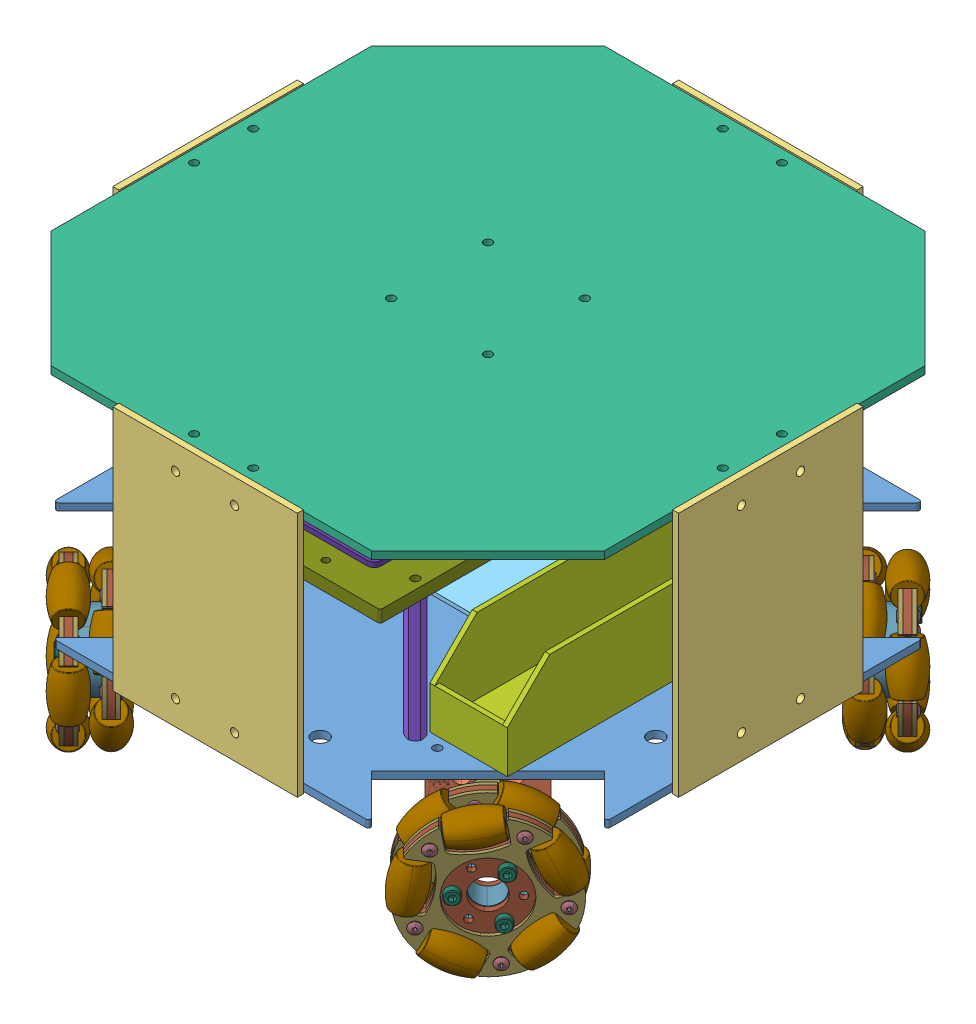
SolidWorks assembly ouijabot, configuration Default. Lengths in mm.
Overall size (259.23 176 257.62).
1225 component instances, 80 part files, 142 mates.
Components (placement in the parent):
- base-1: base [Default] at origin size (228.6 3 228.6)
- motor-mount-pololu-1995-1: motor-mount-pololu-1995 [Default] at (-74.3523 -18.4 78.9485) x (-0.707107 0 -0.707107) z (-0.707107 0 0.707107) size (36.8 36.8 6.5)
- motor-mount-pololu-1995-2: motor-mount-pololu-1995 [Default] at (-78.9485 -18.4 -74.3523) x (0.707107 0 -0.707107) z (-0.707107 0 -0.707107) size (36.8 36.8 6.5)
- motor-mount-pololu-1995-3: motor-mount-pololu-1995 [Default] at (78.9485 -18.4 74.3523) x (-0.707107 0 0.707107) z (0.707107 0 0.707107) size (36.8 36.8 6.5)
- motor-mount-pololu-1995-5: motor-mount-pololu-1995 [Default] at (74.3523 -18.4 -78.9485) x (0.707107 0 0.707107) z (0.707107 0 -0.707107) size (36.8 36.8 6.5)
- motor-pololu-2823-1: motor-pololu-2823 [Default] at (-61.3415 -18.4 33.1633) x (0.707107 0 0.707107) z (-0.707107 0 0.707107) size (36.88 41.23 90.1)
- motor-pololu-2823-2: motor-pololu-2823 [Default] at (33.1633 -18.4 61.3415) x (0.707107 0 -0.707107) z (0.707107 0 0.707107) size (36.88 41.23 90.1)
- motor-pololu-2823-3: motor-pololu-2823 [Default] at (-33.1633 -18.4 -61.3415) x (-0.707107 0 0.707107) z (-0.707107 0 -0.707107) size (36.88 41.23 90.1)
- motor-pololu-2823-4: motor-pololu-2823 [Default] at (61.3415 -18.4 -33.1633) x (-0.707107 0 -0.707107) z (0.707107 0 -0.707107) size (36.88 41.23 90.1)
- standoff-10mm-1: standoff-10mm [94868A166] at (-38 8 0) x (1 0 0) z (0 -1 0) size (4.5 5.2 10.38)
- standoff-10mm-2: standoff-10mm [94868A166] at (38 8 0) x (0.843217 0 -0.537573) z (0 -1 0) size (4.5 5.2 10.38)
- protoboard-1: protoboard [Default] at (0 13 0) size (86.36 1.6 60.96)
- angle-bracket-1: angle-bracket [Default] at (114.3 3 9.025) x (0 0 -1) z (0 1 0) size (6.35 8.71 9.53)
- angle-bracket-2: angle-bracket [Default] at (114.3 3 -15.375) x (0 0 -1) z (0 1 0) size (6.35 8.71 9.53)
- angle-bracket-4: angle-bracket [Default] at (9.025 3 -114.3) x (-1 0 0) z (0 1 0) size (6.35 8.71 9.53)
- angle-bracket-6: angle-bracket [Default] at (-15.375 3 -114.3) x (-1 0 0) z (0 1 0) size (6.35 8.71 9.53)
- angle-bracket-8: angle-bracket [Default] at (-114.3 3 -9.025) x (0 0 1) z (0 1 0) size (6.35 8.71 9.53)
- angle-bracket-10: angle-bracket [Default] at (-114.3 3 15.375) x (0 0 1) z (0 1 0) size (6.35 8.71 9.53)
- angle-bracket-12: angle-bracket [Default] at (-9.025 3 114.3) x (1 0 0) z (0 1 0) size (6.35 8.71 9.53)
- angle-bracket-14: angle-bracket [Default] at (15.375 3 114.3) x (1 0 0) z (0 1 0) size (6.35 8.71 9.53)
- battery-holder-1: battery-holder [Default] at (-65 6.1 0) size (32 35 146)
- battery-holder-2: battery-holder [Default] at (65 6.1 0) size (32 35 146)
- standoff-51mm-1: standoff-51mm [95947A075] at (-44 28.5 74) x (1 0 0) z (0 -1 0) size (6 6.93 51.34)
- standoff-51mm-2: standoff-51mm [95947A075] at (44 28.5 74) x (0.982082 0 -0.188455) z (0 -1 0) size (6 6.93 51.34)
- standoff-51mm-4: standoff-51mm [95947A075] at (44 28.5 -74) x (0.918365 0 -0.395734) z (0 -1 0) size (6 6.93 51.34)
- standoff-51mm-6: standoff-51mm [95947A075] at (-44 28.5 -74) x (0.8 0 -0.6) z (0 -1 0) size (6 6.93 51.34)
- omni-wheel-60mm-1: omni-wheel-60mm [Default] at (-82.2012 -25.4 -82.2012) x (-0.107758 0.98832 0.107758) z (-0.707107 0 -0.707107) size (78.62 80.66 25.5)
  - (Nex) [RB-Nex-75] [14145] 60mm Aluminum Omni Wheel - SolidWorks Model.STEP-1: (Nex) [RB-Nex-75] [14145] 60mm Aluminum Omni Wheel - SolidWorks Model.STEP [Default] at origin size (78.62 80.66 25.5)
    - 60mm90__5______-______________(A__ ).STEP-1: 60mm90__5______-______________(A__ ).STEP [Default] at (0 0 6.25) size (64.79 61.62 13)
      - 60mm90__5______-______________(A__).STEP-1: 60mm90__5______-______________(A__).STEP [Default] at origin size (25 13 13)
        - 60mm90__5______-______(A__).STEP-1: 60mm90__5______-______(A__).STEP [Default] at origin size (18.5 13 13)
        - 60mm90__5______-______-__(A__).STEP-1: 60mm90__5______-______-__(A__).STEP [Default] at (0 23.5 0) x (1 0 0) z (0 -0.978837 -0.204643) size (25 2.5 2.5)
      - 60mm90__5______-______________(A__).STEP-2: 60mm90__5______-______________(A__).STEP [Default] x (0.309017 -0.951057 0) z (0 0 1) size (25 13 13)
        - 60mm90__5______-______(A__).STEP-1: 60mm90__5______-______(A__).STEP [Default] at origin size (18.5 13 13)
        - 60mm90__5______-______-__(A__).STEP-1: 60mm90__5______-______-__(A__).STEP [Default] at (0 23.5 0) x (1 0 0) z (0 -0.978837 -0.204643) size (25 2.5 2.5)
      - 60mm90__5______-______________(A__).STEP-3: 60mm90__5______-______________(A__).STEP [Default] x (-0.809017 -0.587785 0) z (0 0 1) size (25 13 13)
        - 60mm90__5______-______(A__).STEP-1: 60mm90__5______-______(A__).STEP [Default] at origin size (18.5 13 13)
        - 60mm90__5______-______-__(A__).STEP-1: 60mm90__5______-______-__(A__).STEP [Default] at (0 23.5 0) x (1 0 0) z (0 -0.978837 -0.204643) size (25 2.5 2.5)
      - 60mm90__5______-______________(A__).STEP-4: 60mm90__5______-______________(A__).STEP [Default] x (-0.809017 0.587785 0) z (0 0 1) size (25 13 13)
        - 60mm90__5______-______(A__).STEP-1: 60mm90__5______-______(A__).STEP [Default] at origin size (18.5 13 13)
        - 60mm90__5______-______-__(A__).STEP-1: 60mm90__5______-______-__(A__).STEP [Default] at (0 23.5 0) x (1 0 0) z (0 -0.978837 -0.204643) size (25 2.5 2.5)
      - 60mm90__5______-______________(A__).STEP-5: 60mm90__5______-______________(A__).STEP [Default] x (0.309017 0.951057 0) z (0 0 1) size (25 13 13)
        - 60mm90__5______-______(A__).STEP-1: 60mm90__5______-______(A__).STEP [Default] at origin size (18.5 13 13)
        - 60mm90__5______-______-__(A__).STEP-1: 60mm90__5______-______-__(A__).STEP [Default] at (0 23.5 0) x (1 0 0) z (0 -0.978837 -0.204643) size (25 2.5 2.5)
      - 60mm90__5______-____________(A__).STEP-1: 60mm90__5______-____________(A__).STEP [Default] at origin size (56.91 55.07 2.5)
      - 60mm90__5______-__________(A__).STEP-1: 60mm90__5______-__________(A__).STEP [Default] at (0 0 2) size (56.91 55.07 1.5)
      - 60mm90__5______-__________(A__).STEP-2: 60mm90__5______-__________(A__).STEP [Default] at (0 0 -2) size (56.91 55.07 1.5)
      - ____3X5.STEP-1: ____3X5.STEP [Default] at (-14.1068 19.4164 -10.9942) x (1 0 0) z (0 -1 0) size (4.8 7.01 4.8)
      - ____3X5.STEP-2: ____3X5.STEP [Default] at (14.1068 19.4164 -10.9942) x (0.309017 -0.951057 0) z (-0.951057 -0.309017 0) size (4.8 7.01 4.8)
      - ____3X5.STEP-3: ____3X5.STEP [Default] at (22.8254 -7.4164 -10.9942) x (-0.809017 -0.587785 0) z (-0.587785 0.809017 0) size (4.8 7.01 4.8)
      - ____3X5.STEP-4: ____3X5.STEP [Default] at (0 -24 -10.9942) x (-0.809017 0.587785 0) z (0.587785 0.809017 0) size (4.8 7.01 4.8)
      - ____3X5.STEP-5: ____3X5.STEP [Default] at (-22.8254 -7.4164 -10.9942) x (0.309017 0.951057 0) z (0.951057 -0.309017 0) size (4.8 7.01 4.8)
    - 60mm90__5______-______________(A__ ).STEP-2: 60mm90__5______-______________(A__ ).STEP [Default] at (0 0 -6.25) x (0.309017 0.951057 0) z (0 0 -1) size (64.79 61.62 13)
      - 60mm90__5______-______________(A__).STEP-1: 60mm90__5______-______________(A__).STEP [Default] at origin size (25 13 13)
        - 60mm90__5______-______(A__).STEP-1: 60mm90__5______-______(A__).STEP [Default] at origin size (18.5 13 13)
        - 60mm90__5______-______-__(A__).STEP-1: 60mm90__5______-______-__(A__).STEP [Default] at (0 23.5 0) x (1 0 0) z (0 -0.978837 -0.204643) size (25 2.5 2.5)
      - 60mm90__5______-______________(A__).STEP-2: 60mm90__5______-______________(A__).STEP [Default] x (0.309017 -0.951057 0) z (0 0 1) size (25 13 13)
        - 60mm90__5______-______(A__).STEP-1: 60mm90__5______-______(A__).STEP [Default] at origin size (18.5 13 13)
        - 60mm90__5______-______-__(A__).STEP-1: 60mm90__5______-______-__(A__).STEP [Default] at (0 23.5 0) x (1 0 0) z (0 -0.978837 -0.204643) size (25 2.5 2.5)
      - 60mm90__5______-______________(A__).STEP-3: 60mm90__5______-______________(A__).STEP [Default] x (-0.809017 -0.587785 0) z (0 0 1) size (25 13 13)
        - 60mm90__5______-______(A__).STEP-1: 60mm90__5______-______(A__).STEP [Default] at origin size (18.5 13 13)
        - 60mm90__5______-______-__(A__).STEP-1: 60mm90__5______-______-__(A__).STEP [Default] at (0 23.5 0) x (1 0 0) z (0 -0.978837 -0.204643) size (25 2.5 2.5)
      - 60mm90__5______-______________(A__).STEP-4: 60mm90__5______-______________(A__).STEP [Default] x (-0.809017 0.587785 0) z (0 0 1) size (25 13 13)
        - 60mm90__5______-______(A__).STEP-1: 60mm90__5______-______(A__).STEP [Default] at origin size (18.5 13 13)
        - 60mm90__5______-______-__(A__).STEP-1: 60mm90__5______-______-__(A__).STEP [Default] at (0 23.5 0) x (1 0 0) z (0 -0.978837 -0.204643) size (25 2.5 2.5)
      - 60mm90__5______-______________(A__).STEP-5: 60mm90__5______-______________(A__).STEP [Default] x (0.309017 0.951057 0) z (0 0 1) size (25 13 13)
        - 60mm90__5______-______(A__).STEP-1: 60mm90__5______-______(A__).STEP [Default] at origin size (18.5 13 13)
        - 60mm90__5______-______-__(A__).STEP-1: 60mm90__5______-______-__(A__).STEP [Default] at (0 23.5 0) x (1 0 0) z (0 -0.978837 -0.204643) size (25 2.5 2.5)
      - 60mm90__5______-____________(A__).STEP-1: 60mm90__5______-____________(A__).STEP [Default] at origin size (56.91 55.07 2.5)
      - 60mm90__5______-__________(A__).STEP-1: 60mm90__5______-__________(A__).STEP [Default] at (0 0 2) size (56.91 55.07 1.5)
      - 60mm90__5______-__________(A__).STEP-2: 60mm90__5______-__________(A__).STEP [Default] at (0 0 -2) size (56.91 55.07 1.5)
      - ____3X5.STEP-1: ____3X5.STEP [Default] at (-14.1068 19.4164 -10.9942) x (1 0 0) z (0 -1 0) size (4.8 7.01 4.8)
      - ____3X5.STEP-2: ____3X5.STEP [Default] at (14.1068 19.4164 -10.9942) x (0.309017 -0.951057 0) z (-0.951057 -0.309017 0) size (4.8 7.01 4.8)
      - ____3X5.STEP-3: ____3X5.STEP [Default] at (22.8254 -7.4164 -10.9942) x (-0.809017 -0.587785 0) z (-0.587785 0.809017 0) size (4.8 7.01 4.8)
      - ____3X5.STEP-4: ____3X5.STEP [Default] at (0 -24 -10.9942) x (-0.809017 0.587785 0) z (0.587785 0.809017 0) size (4.8 7.01 4.8)
      - ____3X5.STEP-5: ____3X5.STEP [Default] at (-22.8254 -7.4164 -10.9942) x (0.309017 0.951057 0) z (0.951057 -0.309017 0) size (4.8 7.01 4.8)
    - 60mm90__5______-__________(A__)-0.STEP-1: 60mm90__5______-__________(A__)-0.STEP [Default] x (0.994522 0.104528 0) z (0 0 1) size (28 28 10)
    - __________(M3X20).STEP-1: __________(M3X20).STEP [Default] at (-1.0975 10.4425 7.5) x (0.905128 0.425139 0) z (0.425139 -0.905128 0) size (5.5 21 5.5)
    - __________(M3X20).STEP-2: __________(M3X20).STEP [Default] at (-8.4947 -6.1717 7.5) x (-0.820745 0.571294 0) z (0.571294 0.820745 0) size (5.5 21 5.5)
    - __________(M3X20).STEP-3: __________(M3X20).STEP [Default] at (9.5922 -4.2707 7.5) x (-0.084383 -0.996433 0) z (-0.996433 0.084383 0) size (5.5 21 5.5)
- omni-wheel-60mm-2: omni-wheel-60mm [Default] at (82.2012 -25.4 -82.2012) x (-0.276059 0.920643 -0.276059) z (0.707107 0 -0.707107) size (78.62 80.66 25.5)
  - (Nex) [RB-Nex-75] [14145] 60mm Aluminum Omni Wheel - SolidWorks Model.STEP-1: (Nex) [RB-Nex-75] [14145] 60mm Aluminum Omni Wheel - SolidWorks Model.STEP [Default] at origin size (78.62 80.66 25.5)
    - 60mm90__5______-______________(A__ ).STEP-1: 60mm90__5______-______________(A__ ).STEP [Default] at (0 0 6.25) size (64.79 61.62 13)
      - 60mm90__5______-______________(A__).STEP-1: 60mm90__5______-______________(A__).STEP [Default] at origin size (25 13 13)
        - 60mm90__5______-______(A__).STEP-1: 60mm90__5______-______(A__).STEP [Default] at origin size (18.5 13 13)
        - 60mm90__5______-______-__(A__).STEP-1: 60mm90__5______-______-__(A__).STEP [Default] at (0 23.5 0) x (1 0 0) z (0 -0.978837 -0.204643) size (25 2.5 2.5)
      - 60mm90__5______-______________(A__).STEP-2: 60mm90__5______-______________(A__).STEP [Default] x (0.309017 -0.951057 0) z (0 0 1) size (25 13 13)
        - 60mm90__5______-______(A__).STEP-1: 60mm90__5______-______(A__).STEP [Default] at origin size (18.5 13 13)
        - 60mm90__5______-______-__(A__).STEP-1: 60mm90__5______-______-__(A__).STEP [Default] at (0 23.5 0) x (1 0 0) z (0 -0.978837 -0.204643) size (25 2.5 2.5)
      - 60mm90__5______-______________(A__).STEP-3: 60mm90__5______-______________(A__).STEP [Default] x (-0.809017 -0.587785 0) z (0 0 1) size (25 13 13)
        - 60mm90__5______-______(A__).STEP-1: 60mm90__5______-______(A__).STEP [Default] at origin size (18.5 13 13)
        - 60mm90__5______-______-__(A__).STEP-1: 60mm90__5______-______-__(A__).STEP [Default] at (0 23.5 0) x (1 0 0) z (0 -0.978837 -0.204643) size (25 2.5 2.5)
      - 60mm90__5______-______________(A__).STEP-4: 60mm90__5______-______________(A__).STEP [Default] x (-0.809017 0.587785 0) z (0 0 1) size (25 13 13)
        - 60mm90__5______-______(A__).STEP-1: 60mm90__5______-______(A__).STEP [Default] at origin size (18.5 13 13)
        - 60mm90__5______-______-__(A__).STEP-1: 60mm90__5______-______-__(A__).STEP [Default] at (0 23.5 0) x (1 0 0) z (0 -0.978837 -0.204643) size (25 2.5 2.5)
      - 60mm90__5______-______________(A__).STEP-5: 60mm90__5______-______________(A__).STEP [Default] x (0.309017 0.951057 0) z (0 0 1) size (25 13 13)
        - 60mm90__5______-______(A__).STEP-1: 60mm90__5______-______(A__).STEP [Default] at origin size (18.5 13 13)
        - 60mm90__5______-______-__(A__).STEP-1: 60mm90__5______-______-__(A__).STEP [Default] at (0 23.5 0) x (1 0 0) z (0 -0.978837 -0.204643) size (25 2.5 2.5)
      - 60mm90__5______-____________(A__).STEP-1: 60mm90__5______-____________(A__).STEP [Default] at origin size (56.91 55.07 2.5)
      - 60mm90__5______-__________(A__).STEP-1: 60mm90__5______-__________(A__).STEP [Default] at (0 0 2) size (56.91 55.07 1.5)
      - 60mm90__5______-__________(A__).STEP-2: 60mm90__5______-__________(A__).STEP [Default] at (0 0 -2) size (56.91 55.07 1.5)
      - ____3X5.STEP-1: ____3X5.STEP [Default] at (-14.1068 19.4164 -10.9942) x (1 0 0) z (0 -1 0) size (4.8 7.01 4.8)
      - ____3X5.STEP-2: ____3X5.STEP [Default] at (14.1068 19.4164 -10.9942) x (0.309017 -0.951057 0) z (-0.951057 -0.309017 0) size (4.8 7.01 4.8)
      - ____3X5.STEP-3: ____3X5.STEP [Default] at (22.8254 -7.4164 -10.9942) x (-0.809017 -0.587785 0) z (-0.587785 0.809017 0) size (4.8 7.01 4.8)
      - ____3X5.STEP-4: ____3X5.STEP [Default] at (0 -24 -10.9942) x (-0.809017 0.587785 0) z (0.587785 0.809017 0) size (4.8 7.01 4.8)
      - ____3X5.STEP-5: ____3X5.STEP [Default] at (-22.8254 -7.4164 -10.9942) x (0.309017 0.951057 0) z (0.951057 -0.309017 0) size (4.8 7.01 4.8)
    - 60mm90__5______-______________(A__ ).STEP-2: 60mm90__5______-______________(A__ ).STEP [Default] at (0 0 -6.25) x (0.309017 0.951057 0) z (0 0 -1) size (64.79 61.62 13)
      - 60mm90__5______-______________(A__).STEP-1: 60mm90__5______-______________(A__).STEP [Default] at origin size (25 13 13)
        - 60mm90__5______-______(A__).STEP-1: 60mm90__5______-______(A__).STEP [Default] at origin size (18.5 13 13)
        - 60mm90__5______-______-__(A__).STEP-1: 60mm90__5______-______-__(A__).STEP [Default] at (0 23.5 0) x (1 0 0) z (0 -0.978837 -0.204643) size (25 2.5 2.5)
      - 60mm90__5______-______________(A__).STEP-2: 60mm90__5______-______________(A__).STEP [Default] x (0.309017 -0.951057 0) z (0 0 1) size (25 13 13)
        - 60mm90__5______-______(A__).STEP-1: 60mm90__5______-______(A__).STEP [Default] at origin size (18.5 13 13)
        - 60mm90__5______-______-__(A__).STEP-1: 60mm90__5______-______-__(A__).STEP [Default] at (0 23.5 0) x (1 0 0) z (0 -0.978837 -0.204643) size (25 2.5 2.5)
      - 60mm90__5______-______________(A__).STEP-3: 60mm90__5______-______________(A__).STEP [Default] x (-0.809017 -0.587785 0) z (0 0 1) size (25 13 13)
        - 60mm90__5______-______(A__).STEP-1: 60mm90__5______-______(A__).STEP [Default] at origin size (18.5 13 13)
        - 60mm90__5______-______-__(A__).STEP-1: 60mm90__5______-______-__(A__).STEP [Default] at (0 23.5 0) x (1 0 0) z (0 -0.978837 -0.204643) size (25 2.5 2.5)
      - 60mm90__5______-______________(A__).STEP-4: 60mm90__5______-______________(A__).STEP [Default] x (-0.809017 0.587785 0) z (0 0 1) size (25 13 13)
        - 60mm90__5______-______(A__).STEP-1: 60mm90__5______-______(A__).STEP [Default] at origin size (18.5 13 13)
        - 60mm90__5______-______-__(A__).STEP-1: 60mm90__5______-______-__(A__).STEP [Default] at (0 23.5 0) x (1 0 0) z (0 -0.978837 -0.204643) size (25 2.5 2.5)
      - 60mm90__5______-______________(A__).STEP-5: 60mm90__5______-______________(A__).STEP [Default] x (0.309017 0.951057 0) z (0 0 1) size (25 13 13)
        - 60mm90__5______-______(A__).STEP-1: 60mm90__5______-______(A__).STEP [Default] at origin size (18.5 13 13)
        - 60mm90__5______-______-__(A__).STEP-1: 60mm90__5______-______-__(A__).STEP [Default] at (0 23.5 0) x (1 0 0) z (0 -0.978837 -0.204643) size (25 2.5 2.5)
      - 60mm90__5______-____________(A__).STEP-1: 60mm90__5______-____________(A__).STEP [Default] at origin size (56.91 55.07 2.5)
      - 60mm90__5______-__________(A__).STEP-1: 60mm90__5______-__________(A__).STEP [Default] at (0 0 2) size (56.91 55.07 1.5)
      - 60mm90__5______-__________(A__).STEP-2: 60mm90__5______-__________(A__).STEP [Default] at (0 0 -2) size (56.91 55.07 1.5)
      - ____3X5.STEP-1: ____3X5.STEP [Default] at (-14.1068 19.4164 -10.9942) x (1 0 0) z (0 -1 0) size (4.8 7.01 4.8)
      - ____3X5.STEP-2: ____3X5.STEP [Default] at (14.1068 19.4164 -10.9942) x (0.309017 -0.951057 0) z (-0.951057 -0.309017 0) size (4.8 7.01 4.8)
      - ____3X5.STEP-3: ____3X5.STEP [Default] at (22.8254 -7.4164 -10.9942) x (-0.809017 -0.587785 0) z (-0.587785 0.809017 0) size (4.8 7.01 4.8)
      - ____3X5.STEP-4: ____3X5.STEP [Default] at (0 -24 -10.9942) x (-0.809017 0.587785 0) z (0.587785 0.809017 0) size (4.8 7.01 4.8)
      - ____3X5.STEP-5: ____3X5.STEP [Default] at (-22.8254 -7.4164 -10.9942) x (0.309017 0.951057 0) z (0.951057 -0.309017 0) size (4.8 7.01 4.8)
    - 60mm90__5______-__________(A__)-0.STEP-1: 60mm90__5______-__________(A__)-0.STEP [Default] x (0.994522 0.104528 0) z (0 0 1) size (28 28 10)
    - __________(M3X20).STEP-1: __________(M3X20).STEP [Default] at (-1.0975 10.4425 7.5) x (0.905128 0.425139 0) z (0.425139 -0.905128 0) size (5.5 21 5.5)
    - __________(M3X20).STEP-2: __________(M3X20).STEP [Default] at (-8.4947 -6.1717 7.5) x (-0.820745 0.571294 0) z (0.571294 0.820745 0) size (5.5 21 5.5)
    - __________(M3X20).STEP-3: __________(M3X20).STEP [Default] at (9.5922 -4.2707 7.5) x (-0.084383 -0.996433 0) z (-0.996433 0.084383 0) size (5.5 21 5.5)
- omni-wheel-60mm-4: omni-wheel-60mm [Default] at (82.2012 -25.4 82.2012) x (0.107758 0.98832 -0.107758) z (0.707107 0 0.707107) size (78.62 80.66 25.5)
  - (Nex) [RB-Nex-75] [14145] 60mm Aluminum Omni Wheel - SolidWorks Model.STEP-1: (Nex) [RB-Nex-75] [14145] 60mm Aluminum Omni Wheel - SolidWorks Model.STEP [Default] at origin size (78.62 80.66 25.5)
    - 60mm90__5______-______________(A__ ).STEP-1: 60mm90__5______-______________(A__ ).STEP [Default] at (0 0 6.25) size (64.79 61.62 13)
      - 60mm90__5______-______________(A__).STEP-1: 60mm90__5______-______________(A__).STEP [Default] at origin size (25 13 13)
        - 60mm90__5______-______(A__).STEP-1: 60mm90__5______-______(A__).STEP [Default] at origin size (18.5 13 13)
        - 60mm90__5______-______-__(A__).STEP-1: 60mm90__5______-______-__(A__).STEP [Default] at (0 23.5 0) x (1 0 0) z (0 -0.978837 -0.204643) size (25 2.5 2.5)
      - 60mm90__5______-______________(A__).STEP-2: 60mm90__5______-______________(A__).STEP [Default] x (0.309017 -0.951057 0) z (0 0 1) size (25 13 13)
        - 60mm90__5______-______(A__).STEP-1: 60mm90__5______-______(A__).STEP [Default] at origin size (18.5 13 13)
        - 60mm90__5______-______-__(A__).STEP-1: 60mm90__5______-______-__(A__).STEP [Default] at (0 23.5 0) x (1 0 0) z (0 -0.978837 -0.204643) size (25 2.5 2.5)
      - 60mm90__5______-______________(A__).STEP-3: 60mm90__5______-______________(A__).STEP [Default] x (-0.809017 -0.587785 0) z (0 0 1) size (25 13 13)
        - 60mm90__5______-______(A__).STEP-1: 60mm90__5______-______(A__).STEP [Default] at origin size (18.5 13 13)
        - 60mm90__5______-______-__(A__).STEP-1: 60mm90__5______-______-__(A__).STEP [Default] at (0 23.5 0) x (1 0 0) z (0 -0.978837 -0.204643) size (25 2.5 2.5)
      - 60mm90__5______-______________(A__).STEP-4: 60mm90__5______-______________(A__).STEP [Default] x (-0.809017 0.587785 0) z (0 0 1) size (25 13 13)
        - 60mm90__5______-______(A__).STEP-1: 60mm90__5______-______(A__).STEP [Default] at origin size (18.5 13 13)
        - 60mm90__5______-______-__(A__).STEP-1: 60mm90__5______-______-__(A__).STEP [Default] at (0 23.5 0) x (1 0 0) z (0 -0.978837 -0.204643) size (25 2.5 2.5)
      - 60mm90__5______-______________(A__).STEP-5: 60mm90__5______-______________(A__).STEP [Default] x (0.309017 0.951057 0) z (0 0 1) size (25 13 13)
        - 60mm90__5______-______(A__).STEP-1: 60mm90__5______-______(A__).STEP [Default] at origin size (18.5 13 13)
        - 60mm90__5______-______-__(A__).STEP-1: 60mm90__5______-______-__(A__).STEP [Default] at (0 23.5 0) x (1 0 0) z (0 -0.978837 -0.204643) size (25 2.5 2.5)
      - 60mm90__5______-____________(A__).STEP-1: 60mm90__5______-____________(A__).STEP [Default] at origin size (56.91 55.07 2.5)
      - 60mm90__5______-__________(A__).STEP-1: 60mm90__5______-__________(A__).STEP [Default] at (0 0 2) size (56.91 55.07 1.5)
      - 60mm90__5______-__________(A__).STEP-2: 60mm90__5______-__________(A__).STEP [Default] at (0 0 -2) size (56.91 55.07 1.5)
      - ____3X5.STEP-1: ____3X5.STEP [Default] at (-14.1068 19.4164 -10.9942) x (1 0 0) z (0 -1 0) size (4.8 7.01 4.8)
      - ____3X5.STEP-2: ____3X5.STEP [Default] at (14.1068 19.4164 -10.9942) x (0.309017 -0.951057 0) z (-0.951057 -0.309017 0) size (4.8 7.01 4.8)
      - ____3X5.STEP-3: ____3X5.STEP [Default] at (22.8254 -7.4164 -10.9942) x (-0.809017 -0.587785 0) z (-0.587785 0.809017 0) size (4.8 7.01 4.8)
      - ____3X5.STEP-4: ____3X5.STEP [Default] at (0 -24 -10.9942) x (-0.809017 0.587785 0) z (0.587785 0.809017 0) size (4.8 7.01 4.8)
      - ____3X5.STEP-5: ____3X5.STEP [Default] at (-22.8254 -7.4164 -10.9942) x (0.309017 0.951057 0) z (0.951057 -0.309017 0) size (4.8 7.01 4.8)
    - 60mm90__5______-______________(A__ ).STEP-2: 60mm90__5______-______________(A__ ).STEP [Default] at (0 0 -6.25) x (0.309017 0.951057 0) z (0 0 -1) size (64.79 61.62 13)
      - 60mm90__5______-______________(A__).STEP-1: 60mm90__5______-______________(A__).STEP [Default] at origin size (25 13 13)
        - 60mm90__5______-______(A__).STEP-1: 60mm90__5______-______(A__).STEP [Default] at origin size (18.5 13 13)
        - 60mm90__5______-______-__(A__).STEP-1: 60mm90__5______-______-__(A__).STEP [Default] at (0 23.5 0) x (1 0 0) z (0 -0.978837 -0.204643) size (25 2.5 2.5)
      - 60mm90__5______-______________(A__).STEP-2: 60mm90__5______-______________(A__).STEP [Default] x (0.309017 -0.951057 0) z (0 0 1) size (25 13 13)
        - 60mm90__5______-______(A__).STEP-1: 60mm90__5______-______(A__).STEP [Default] at origin size (18.5 13 13)
        - 60mm90__5______-______-__(A__).STEP-1: 60mm90__5______-______-__(A__).STEP [Default] at (0 23.5 0) x (1 0 0) z (0 -0.978837 -0.204643) size (25 2.5 2.5)
      - 60mm90__5______-______________(A__).STEP-3: 60mm90__5______-______________(A__).STEP [Default] x (-0.809017 -0.587785 0) z (0 0 1) size (25 13 13)
        - 60mm90__5______-______(A__).STEP-1: 60mm90__5______-______(A__).STEP [Default] at origin size (18.5 13 13)
        - 60mm90__5______-______-__(A__).STEP-1: 60mm90__5______-______-__(A__).STEP [Default] at (0 23.5 0) x (1 0 0) z (0 -0.978837 -0.204643) size (25 2.5 2.5)
      - 60mm90__5______-______________(A__).STEP-4: 60mm90__5______-______________(A__).STEP [Default] x (-0.809017 0.587785 0) z (0 0 1) size (25 13 13)
        - 60mm90__5______-______(A__).STEP-1: 60mm90__5______-______(A__).STEP [Default] at origin size (18.5 13 13)
        - 60mm90__5______-______-__(A__).STEP-1: 60mm90__5______-______-__(A__).STEP [Default] at (0 23.5 0) x (1 0 0) z (0 -0.978837 -0.204643) size (25 2.5 2.5)
      - 60mm90__5______-______________(A__).STEP-5: 60mm90__5______-______________(A__).STEP [Default] x (0.309017 0.951057 0) z (0 0 1) size (25 13 13)
        - 60mm90__5______-______(A__).STEP-1: 60mm90__5______-______(A__).STEP [Default] at origin size (18.5 13 13)
        - 60mm90__5______-______-__(A__).STEP-1: 60mm90__5______-______-__(A__).STEP [Default] at (0 23.5 0) x (1 0 0) z (0 -0.978837 -0.204643) size (25 2.5 2.5)
      - 60mm90__5______-____________(A__).STEP-1: 60mm90__5______-____________(A__).STEP [Default] at origin size (56.91 55.07 2.5)
      - 60mm90__5______-__________(A__).STEP-1: 60mm90__5______-__________(A__).STEP [Default] at (0 0 2) size (56.91 55.07 1.5)
      - 60mm90__5______-__________(A__).STEP-2: 60mm90__5______-__________(A__).STEP [Default] at (0 0 -2) size (56.91 55.07 1.5)
      - ____3X5.STEP-1: ____3X5.STEP [Default] at (-14.1068 19.4164 -10.9942) x (1 0 0) z (0 -1 0) size (4.8 7.01 4.8)
      - ____3X5.STEP-2: ____3X5.STEP [Default] at (14.1068 19.4164 -10.9942) x (0.309017 -0.951057 0) z (-0.951057 -0.309017 0) size (4.8 7.01 4.8)
      - ____3X5.STEP-3: ____3X5.STEP [Default] at (22.8254 -7.4164 -10.9942) x (-0.809017 -0.587785 0) z (-0.587785 0.809017 0) size (4.8 7.01 4.8)
      - ____3X5.STEP-4: ____3X5.STEP [Default] at (0 -24 -10.9942) x (-0.809017 0.587785 0) z (0.587785 0.809017 0) size (4.8 7.01 4.8)
      - ____3X5.STEP-5: ____3X5.STEP [Default] at (-22.8254 -7.4164 -10.9942) x (0.309017 0.951057 0) z (0.951057 -0.309017 0) size (4.8 7.01 4.8)
    - 60mm90__5______-__________(A__)-0.STEP-1: 60mm90__5______-__________(A__)-0.STEP [Default] x (0.994522 0.104528 0) z (0 0 1) size (28 28 10)
    - __________(M3X20).STEP-1: __________(M3X20).STEP [Default] at (-1.0975 10.4425 7.5) x (0.905128 0.425139 0) z (0.425139 -0.905128 0) size (5.5 21 5.5)
    - __________(M3X20).STEP-2: __________(M3X20).STEP [Default] at (-8.4947 -6.1717 7.5) x (-0.820745 0.571294 0) z (0.571294 0.820745 0) size (5.5 21 5.5)
    - __________(M3X20).STEP-3: __________(M3X20).STEP [Default] at (9.5922 -4.2707 7.5) x (-0.084383 -0.996433 0) z (-0.996433 0.084383 0) size (5.5 21 5.5)
- omni-wheel-60mm-6: omni-wheel-60mm [Default] at (-82.2012 -25.4 82.2012) x (0.373028 0.849529 0.373028) z (-0.707107 0 0.707107) size (78.62 80.66 25.5)
  - (Nex) [RB-Nex-75] [14145] 60mm Aluminum Omni Wheel - SolidWorks Model.STEP-1: (Nex) [RB-Nex-75] [14145] 60mm Aluminum Omni Wheel - SolidWorks Model.STEP [Default] at origin size (78.62 80.66 25.5)
    - 60mm90__5______-______________(A__ ).STEP-1: 60mm90__5______-______________(A__ ).STEP [Default] at (0 0 6.25) size (64.79 61.62 13)
      - 60mm90__5______-______________(A__).STEP-1: 60mm90__5______-______________(A__).STEP [Default] at origin size (25 13 13)
        - 60mm90__5______-______(A__).STEP-1: 60mm90__5______-______(A__).STEP [Default] at origin size (18.5 13 13)
        - 60mm90__5______-______-__(A__).STEP-1: 60mm90__5______-______-__(A__).STEP [Default] at (0 23.5 0) x (1 0 0) z (0 -0.978837 -0.204643) size (25 2.5 2.5)
      - 60mm90__5______-______________(A__).STEP-2: 60mm90__5______-______________(A__).STEP [Default] x (0.309017 -0.951057 0) z (0 0 1) size (25 13 13)
        - 60mm90__5______-______(A__).STEP-1: 60mm90__5______-______(A__).STEP [Default] at origin size (18.5 13 13)
        - 60mm90__5______-______-__(A__).STEP-1: 60mm90__5______-______-__(A__).STEP [Default] at (0 23.5 0) x (1 0 0) z (0 -0.978837 -0.204643) size (25 2.5 2.5)
      - 60mm90__5______-______________(A__).STEP-3: 60mm90__5______-______________(A__).STEP [Default] x (-0.809017 -0.587785 0) z (0 0 1) size (25 13 13)
        - 60mm90__5______-______(A__).STEP-1: 60mm90__5______-______(A__).STEP [Default] at origin size (18.5 13 13)
        - 60mm90__5______-______-__(A__).STEP-1: 60mm90__5______-______-__(A__).STEP [Default] at (0 23.5 0) x (1 0 0) z (0 -0.978837 -0.204643) size (25 2.5 2.5)
      - 60mm90__5______-______________(A__).STEP-4: 60mm90__5______-______________(A__).STEP [Default] x (-0.809017 0.587785 0) z (0 0 1) size (25 13 13)
        - 60mm90__5______-______(A__).STEP-1: 60mm90__5______-______(A__).STEP [Default] at origin size (18.5 13 13)
        - 60mm90__5______-______-__(A__).STEP-1: 60mm90__5______-______-__(A__).STEP [Default] at (0 23.5 0) x (1 0 0) z (0 -0.978837 -0.204643) size (25 2.5 2.5)
      - 60mm90__5______-______________(A__).STEP-5: 60mm90__5______-______________(A__).STEP [Default] x (0.309017 0.951057 0) z (0 0 1) size (25 13 13)
        - 60mm90__5______-______(A__).STEP-1: 60mm90__5______-______(A__).STEP [Default] at origin size (18.5 13 13)
        - 60mm90__5______-______-__(A__).STEP-1: 60mm90__5______-______-__(A__).STEP [Default] at (0 23.5 0) x (1 0 0) z (0 -0.978837 -0.204643) size (25 2.5 2.5)
      - 60mm90__5______-____________(A__).STEP-1: 60mm90__5______-____________(A__).STEP [Default] at origin size (56.91 55.07 2.5)
      - 60mm90__5______-__________(A__).STEP-1: 60mm90__5______-__________(A__).STEP [Default] at (0 0 2) size (56.91 55.07 1.5)
      - 60mm90__5______-__________(A__).STEP-2: 60mm90__5______-__________(A__).STEP [Default] at (0 0 -2) size (56.91 55.07 1.5)
      - ____3X5.STEP-1: ____3X5.STEP [Default] at (-14.1068 19.4164 -10.9942) x (1 0 0) z (0 -1 0) size (4.8 7.01 4.8)
      - ____3X5.STEP-2: ____3X5.STEP [Default] at (14.1068 19.4164 -10.9942) x (0.309017 -0.951057 0) z (-0.951057 -0.309017 0) size (4.8 7.01 4.8)
      - ____3X5.STEP-3: ____3X5.STEP [Default] at (22.8254 -7.4164 -10.9942) x (-0.809017 -0.587785 0) z (-0.587785 0.809017 0) size (4.8 7.01 4.8)
      - ____3X5.STEP-4: ____3X5.STEP [Default] at (0 -24 -10.9942) x (-0.809017 0.587785 0) z (0.587785 0.809017 0) size (4.8 7.01 4.8)
      - ____3X5.STEP-5: ____3X5.STEP [Default] at (-22.8254 -7.4164 -10.9942) x (0.309017 0.951057 0) z (0.951057 -0.309017 0) size (4.8 7.01 4.8)
    - 60mm90__5______-______________(A__ ).STEP-2: 60mm90__5______-______________(A__ ).STEP [Default] at (0 0 -6.25) x (0.309017 0.951057 0) z (0 0 -1) size (64.79 61.62 13)
      - 60mm90__5______-______________(A__).STEP-1: 60mm90__5______-______________(A__).STEP [Default] at origin size (25 13 13)
        - 60mm90__5______-______(A__).STEP-1: 60mm90__5______-______(A__).STEP [Default] at origin size (18.5 13 13)
        - 60mm90__5______-______-__(A__).STEP-1: 60mm90__5______-______-__(A__).STEP [Default] at (0 23.5 0) x (1 0 0) z (0 -0.978837 -0.204643) size (25 2.5 2.5)
      - 60mm90__5______-______________(A__).STEP-2: 60mm90__5______-______________(A__).STEP [Default] x (0.309017 -0.951057 0) z (0 0 1) size (25 13 13)
        - 60mm90__5______-______(A__).STEP-1: 60mm90__5______-______(A__).STEP [Default] at origin size (18.5 13 13)
        - 60mm90__5______-______-__(A__).STEP-1: 60mm90__5______-______-__(A__).STEP [Default] at (0 23.5 0) x (1 0 0) z (0 -0.978837 -0.204643) size (25 2.5 2.5)
      - 60mm90__5______-______________(A__).STEP-3: 60mm90__5______-______________(A__).STEP [Default] x (-0.809017 -0.587785 0) z (0 0 1) size (25 13 13)
        - 60mm90__5______-______(A__).STEP-1: 60mm90__5______-______(A__).STEP [Default] at origin size (18.5 13 13)
        - 60mm90__5______-______-__(A__).STEP-1: 60mm90__5______-______-__(A__).STEP [Default] at (0 23.5 0) x (1 0 0) z (0 -0.978837 -0.204643) size (25 2.5 2.5)
      - 60mm90__5______-______________(A__).STEP-4: 60mm90__5______-______________(A__).STEP [Default] x (-0.809017 0.587785 0) z (0 0 1) size (25 13 13)
        - 60mm90__5______-______(A__).STEP-1: 60mm90__5______-______(A__).STEP [Default] at origin size (18.5 13 13)
        - 60mm90__5______-______-__(A__).STEP-1: 60mm90__5______-______-__(A__).STEP [Default] at (0 23.5 0) x (1 0 0) z (0 -0.978837 -0.204643) size (25 2.5 2.5)
      - 60mm90__5______-______________(A__).STEP-5: 60mm90__5______-______________(A__).STEP [Default] x (0.309017 0.951057 0) z (0 0 1) size (25 13 13)
        - 60mm90__5______-______(A__).STEP-1: 60mm90__5______-______(A__).STEP [Default] at origin size (18.5 13 13)
        - 60mm90__5______-______-__(A__).STEP-1: 60mm90__5______-______-__(A__).STEP [Default] at (0 23.5 0) x (1 0 0) z (0 -0.978837 -0.204643) size (25 2.5 2.5)
      - 60mm90__5______-____________(A__).STEP-1: 60mm90__5______-____________(A__).STEP [Default] at origin size (56.91 55.07 2.5)
      - 60mm90__5______-__________(A__).STEP-1: 60mm90__5______-__________(A__).STEP [Default] at (0 0 2) size (56.91 55.07 1.5)
      - 60mm90__5______-__________(A__).STEP-2: 60mm90__5______-__________(A__).STEP [Default] at (0 0 -2) size (56.91 55.07 1.5)
      - ____3X5.STEP-1: ____3X5.STEP [Default] at (-14.1068 19.4164 -10.9942) x (1 0 0) z (0 -1 0) size (4.8 7.01 4.8)
      - ____3X5.STEP-2: ____3X5.STEP [Default] at (14.1068 19.4164 -10.9942) x (0.309017 -0.951057 0) z (-0.951057 -0.309017 0) size (4.8 7.01 4.8)
      - ____3X5.STEP-3: ____3X5.STEP [Default] at (22.8254 -7.4164 -10.9942) x (-0.809017 -0.587785 0) z (-0.587785 0.809017 0) size (4.8 7.01 4.8)
      - ____3X5.STEP-4: ____3X5.STEP [Default] at (0 -24 -10.9942) x (-0.809017 0.587785 0) z (0.587785 0.809017 0) size (4.8 7.01 4.8)
      - ____3X5.STEP-5: ____3X5.STEP [Default] at (-22.8254 -7.4164 -10.9942) x (0.309017 0.951057 0) z (0.951057 -0.309017 0) size (4.8 7.01 4.8)
    - 60mm90__5______-__________(A__)-0.STEP-1: 60mm90__5______-__________(A__)-0.STEP [Default] x (0.994522 0.104528 0) z (0 0 1) size (28 28 10)
    - __________(M3X20).STEP-1: __________(M3X20).STEP [Default] at (-1.0975 10.4425 7.5) x (0.905128 0.425139 0) z (0.425139 -0.905128 0) size (5.5 21 5.5)
    - __________(M3X20).STEP-2: __________(M3X20).STEP [Default] at (-8.4947 -6.1717 7.5) x (-0.820745 0.571294 0) z (0.571294 0.820745 0) size (5.5 21 5.5)
    - __________(M3X20).STEP-3: __________(M3X20).STEP [Default] at (9.5922 -4.2707 7.5) x (-0.084383 -0.996433 0) z (-0.996433 0.084383 0) size (5.5 21 5.5)
- level2-plate-1: level2-plate [Default] at (0 54 0) size (96 5 185)
- standoff-10mm-3: standoff-10mm [94868A166] at (-38 64 0) x (1 0 0) z (0 -1 0) size (4.5 5.2 10.38)
- standoff-10mm-4: standoff-10mm [94868A166] at (38 64 0) x (0.982082 0 -0.188455) z (0 -1 0) size (4.5 5.2 10.38)
- protoboard-2: protoboard [Default] at (0 69 0) size (86.36 1.6 60.96)
- raspberry_pi-1: raspberry_pi [Default] at (0 69 61.48) x (0 0 1) z (-1 0 0) size (56 2 85)
- tx2-carrier-orbitty-1: tx2-carrier-orbitty [Default] at (43.5 74 -33.48) x (-1 0 0) z (0 -1 0) size (87.04 52.68 23.65)
  - ASG003_3D_MODEL.step-1: ASG003_3D_MODEL.step [Default] at origin size (87.04 52.68 23.65)
    - R53.step-1: R53.step [Default] at origin size (1.02 0.52 0.36)
      - 870940480.step-1: 870940480.step [Default] at (7.8976 25.146 -1.9516) size (0.16 0.52 0.35)
        - Extruded.step-1: Extruded.step [Default] at origin size (0.16 0.52 0.35)
      - 870940480.step-2: 870940480.step [Default] at (7.0376 25.146 -1.9516) size (0.16 0.52 0.35)
        - Extruded.step-1: Extruded.step [Default] at origin size (0.16 0.52 0.35)
      - 870940640.step-1: 870940640.step [Default] at (7.4676 25.146 -1.9506) size (1.01 0.51 0.36)
        - Extruded-0.step-1: Extruded-0.step [Default] at origin size (1.01 0.51 0.36)
    - R52.step-1: R52.step [Default] at origin size (0.52 1.02 0.36)
      - 870941120.step-1: 870941120.step [Default] at (69.723 24.306 0) size (0.52 0.16 0.35)
        - Extruded-1.step-1: Extruded-1.step [Default] at origin size (0.52 0.16 0.35)
      - 870941120.step-2: 870941120.step [Default] at (69.723 23.446 0) size (0.52 0.16 0.35)
        - Extruded-1.step-1: Extruded-1.step [Default] at origin size (0.52 0.16 0.35)
      - 870941280.step-1: 870941280.step [Default] at (69.723 23.876 0) size (0.51 1.01 0.36)
        - Extruded-2.step-1: Extruded-2.step [Default] at origin size (0.51 1.01 0.36)
    - R40.step-1: R40.step [Default] at origin size (0.52 1.02 0.36)
      - 870941120.step-1: 870941120.step [Default] at (70.739 24.306 0) size (0.52 0.16 0.35)
        - Extruded-1.step-1: Extruded-1.step [Default] at origin size (0.52 0.16 0.35)
      - 870941120.step-2: 870941120.step [Default] at (70.739 23.446 0) size (0.52 0.16 0.35)
        - Extruded-1.step-1: Extruded-1.step [Default] at origin size (0.52 0.16 0.35)
      - 870941280.step-1: 870941280.step [Default] at (70.739 23.876 0) size (0.51 1.01 0.36)
        - Extruded-2.step-1: Extruded-2.step [Default] at origin size (0.51 1.01 0.36)
    - C59.step-1: C59.step [Default] at origin size (1.02 0.52 0.36)
      - 870940480.step-1: 870940480.step [Default] at (34.847 5.588 0) size (0.16 0.52 0.35)
        - Extruded.step-1: Extruded.step [Default] at origin size (0.16 0.52 0.35)
      - 870940480.step-2: 870940480.step [Default] at (33.987 5.588 0) size (0.16 0.52 0.35)
        - Extruded.step-1: Extruded.step [Default] at origin size (0.16 0.52 0.35)
      - 870940640.step-1: 870940640.step [Default] at (34.417 5.588 0) size (1.01 0.51 0.36)
        - Extruded-0.step-1: Extruded-0.step [Default] at origin size (1.01 0.51 0.36)
    - R51.step-1: R51.step [Default] at origin size (2.5 3.5 0.64)
      - 870944960.step-1: 870944960.step [Default] at (16.256 43.688 -2.2356) size (2.5 3.5 0.64)
        - Extruded-3.step-1: Extruded-3.step [Default] at origin size (2.5 3.5 0.64)
    - R14.step-1: R14.step [Default] at origin size (1.02 0.52 0.36)
      - 870940480.step-1: 870940480.step [Default] at (3.888 14.351 0) size (0.16 0.52 0.35)
        - Extruded.step-1: Extruded.step [Default] at origin size (0.16 0.52 0.35)
      - 870940480.step-2: 870940480.step [Default] at (4.748 14.351 0) size (0.16 0.52 0.35)
        - Extruded.step-1: Extruded.step [Default] at origin size (0.16 0.52 0.35)
      - 870940640.step-1: 870940640.step [Default] at (4.318 14.351 0) size (1.01 0.51 0.36)
        - Extruded-0.step-1: Extruded-0.step [Default] at origin size (1.01 0.51 0.36)
    - R13.step-1: R13.step [Default] at origin size (0.52 1.02 0.36)
      - 870941120.step-1: 870941120.step [Default] at (2.032 10.336 0) size (0.52 0.16 0.35)
        - Extruded-1.step-1: Extruded-1.step [Default] at origin size (0.52 0.16 0.35)
      - 870941120.step-2: 870941120.step [Default] at (2.032 9.476 0) size (0.52 0.16 0.35)
        - Extruded-1.step-1: Extruded-1.step [Default] at origin size (0.52 0.16 0.35)
      - 870941280.step-1: 870941280.step [Default] at (2.032 9.906 0) size (0.51 1.01 0.36)
        - Extruded-2.step-1: Extruded-2.step [Default] at origin size (0.51 1.01 0.36)
    - R12.step-1: R12.step [Default] at origin size (0.52 1.02 0.36)
      - 870941120.step-1: 870941120.step [Default] at (7.112 20.017 0) size (0.52 0.16 0.35)
        - Extruded-1.step-1: Extruded-1.step [Default] at origin size (0.52 0.16 0.35)
      - 870941120.step-2: 870941120.step [Default] at (7.112 20.877 0) size (0.52 0.16 0.35)
        - Extruded-1.step-1: Extruded-1.step [Default] at origin size (0.52 0.16 0.35)
      - 870941280.step-1: 870941280.step [Default] at (7.112 20.447 0) size (0.51 1.01 0.36)
        - Extruded-2.step-1: Extruded-2.step [Default] at origin size (0.51 1.01 0.36)
    - D1.step-1: D1.step [Default] at origin size (2.42 2.9 1)
      - SW3dPS-SOT-23.step-1: SW3dPS-SOT-23.step [Default] at (3.683 11.8109 0.498) x (1 0 0) z (0 -1 0) size (2.42 1 2.9)
    - C33.step-1: C33.step [Default] at origin size (2.72 3.52 2.51)
      - 870945120.step-1: 870945120.step [Default] at (19.431 43.688 -4.1006) size (2.7 3.5 2.5)
        - Extruded-4.step-1: Extruded-4.step [Default] at origin size (2.7 3.5 2.5)
      - 870945280.step-1: 870945280.step [Default] at (19.431 45.243 -4.1106) size (2.72 0.41 2.51)
        - Extruded-5.step-1: Extruded-5.step [Default] at origin size (2.72 0.41 2.51)
      - 870945280.step-2: 870945280.step [Default] at (19.431 42.133 -4.1106) size (2.72 0.41 2.51)
        - Extruded-5.step-1: Extruded-5.step [Default] at origin size (2.72 0.41 2.51)
    - C20.step-1: C20.step [Default] at origin size (1.02 0.52 0.36)
      - 870940480.step-1: 870940480.step [Default] at (3.634 9.271 0) size (0.16 0.52 0.35)
        - Extruded.step-1: Extruded.step [Default] at origin size (0.16 0.52 0.35)
      - 870940480.step-2: 870940480.step [Default] at (4.494 9.271 0) size (0.16 0.52 0.35)
        - Extruded.step-1: Extruded.step [Default] at origin size (0.16 0.52 0.35)
      - 870940640.step-1: 870940640.step [Default] at (4.064 9.271 0) size (1.01 0.51 0.36)
        - Extruded-0.step-1: Extruded-0.step [Default] at origin size (1.01 0.51 0.36)
    - C7.step-1: C7.step [Default] at origin size (1.02 0.52 0.36)
      - 870940480.step-1: 870940480.step [Default] at (13.794 4.064 0) size (0.16 0.52 0.35)
        - Extruded.step-1: Extruded.step [Default] at origin size (0.16 0.52 0.35)
      - 870940480.step-2: 870940480.step [Default] at (14.654 4.064 0) size (0.16 0.52 0.35)
        - Extruded.step-1: Extruded.step [Default] at origin size (0.16 0.52 0.35)
      - 870940640.step-1: 870940640.step [Default] at (14.224 4.064 0) size (1.01 0.51 0.36)
        - Extruded-0.step-1: Extruded-0.step [Default] at origin size (1.01 0.51 0.36)
    - U10.step-1: U10.step [Default] at origin size (1.26 2.01 0.91)
      - 870945920.step-1: 870945920.step [Default] at (16.6362 34.3856 -2.6006) size (1.26 2.01 0.91)
        - Extruded-6.step-1: Extruded-6.step [Default] at origin size (1.26 2.01 0.91)
    - U9.step-1: U9.step [Default] at origin size (2.9 1.75 0.99)
      - 870946400.step-1: 870946400.step [Default] at (19.9382 34.2586 -2.6006) size (2.9 1.75 0.99)
        - Extruded-7.step-1: Extruded-7.step [Default] at origin size (2.9 1.75 0.99)
    - U8.step-1: U8.step [Default] at origin size (1.26 2.01 0.91)
      - 870945920.step-1: 870945920.step [Default] at (17.6522 30.9566 -2.6006) size (1.26 2.01 0.91)
